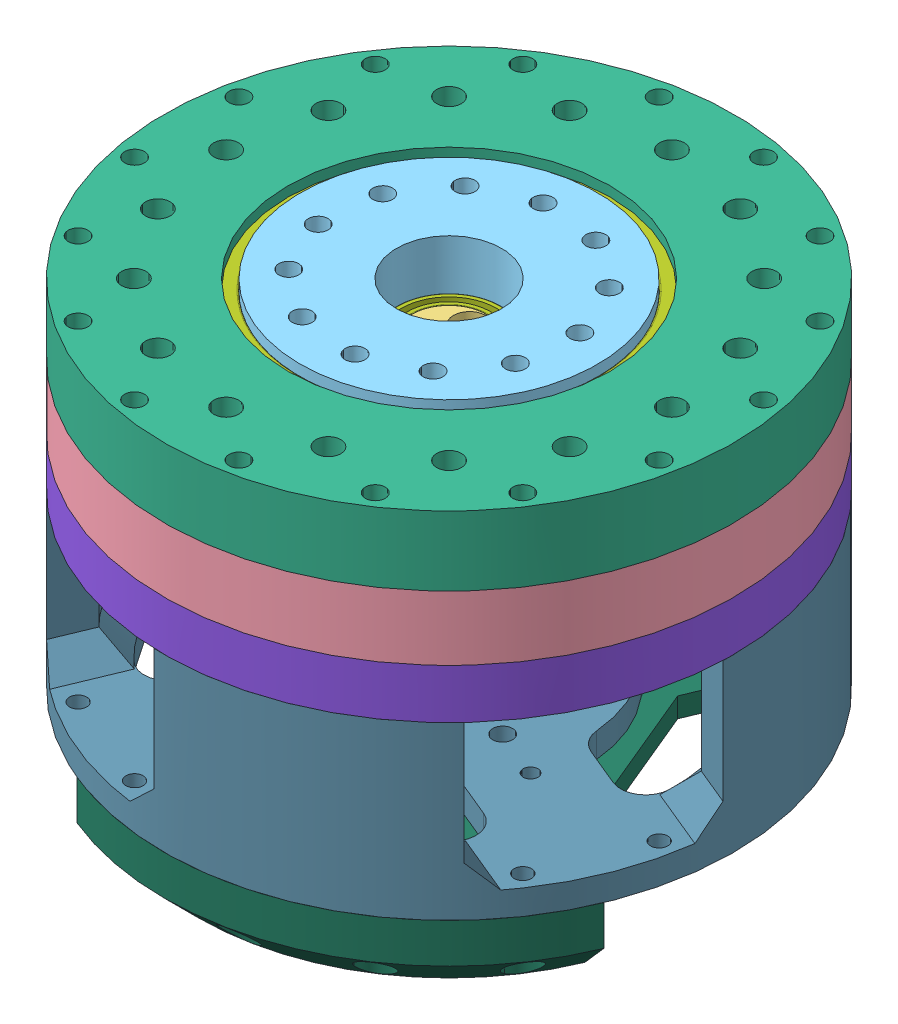
SolidWorks assembly Cycloidal, configuration Default. Lengths in mm.
Overall size (162.63 86.6 162.63).
91 component instances, 15 part files, 83 mates.
Components (placement in the parent):
- motor-X83008S.stp-1: motor-X83008S.stp [Default] at (44.8559 83.3915 132.8566) x (-0.221421 0 -0.975178) z (0 -1 0) (suppressed, hidden)
- Base_Plate-1: Base_Plate [Default] at (47.267 63.2573 89.1587) x (-0.03427 0 0.999413) z (-0.999413 0 -0.03427) size (39.8 11 39.8)
- Eccentric_Shaft-1: Eccentric_Shaft [Default] at (54.4098 67.9165 103.5023) x (-0.999413 0 -0.03427) z (0.03427 0 -0.999413) size (20 17 17)
  - Eccentric_Shaft_bot-1: Eccentric_Shaft_bot [Default] at (7.6302 12.3409 14.0904) x (1 0 0) z (0 0 -1) size (17 6 17)
  - Eccentric_Shaft_bot-2: Eccentric_Shaft_bot [Default] at (7.6302 12.3409 14.0904) x (-1 0 0) z (0 0 -1) size (17 6 17)
  - Eccentric_Shaft_top-1: Eccentric_Shaft_top [Default] at (7.6302 18.3409 14.0904) x (-1 0 0) z (0 0 -1) size (17 5 17)
- Ring_Pin_Housing-1: Ring_Pin_Housing [Default] at (47.267 74.2573 89.1587) x (0.707107 0 -0.707107) z (0.707107 0 0.707107) size (115 13 115)
- Output_Shaft-1: Output_Shaft [Default] at (47.267 87.2573 89.1587) x (0.353379 0 -0.93548) z (0.93548 0 0.353379) size (70 14 70)
- Cover-1: Cover [Default] at (47.267 87.2573 89.1587) x (0.707107 0 -0.707107) z (0.707107 0 0.707107) size (115 14.4 115)
- radial ball bearing_68_iso-39: radial ball bearing_68_iso [ISO 15 RBB - 1860 - 32,SI,NC,32_68] at (47.267 94.2573 89.1587) x (0 1 0) z (-0.131235 0 0.991351) size (10 78 78)
- radial ball bearing_68_iso-40: radial ball bearing_68_iso [ISO 15 RBB - 1840 - 32,SI,NC,32_68] at (47.267 70.7573 89.1587) x (0 1 0) z (0.001003 0 0.999999) size (7 52 52)
- Base_plate_2-1: Base_plate_2 [Default] at (47.267 64.2573 89.1587) x (0.707107 0 -0.707107) z (0.707107 0 0.707107) size (115 10 115)
- m13_bearing-31: m13_bearing [Default] at (-10.7414 95.4081 67.0593) x (0.227678 0 0.973736) z (0.973736 0 -0.227678) size (13 16 13)
  - m6-1: m6 [Default] at (8.4921 2.5508 14.8914) size (6 16 6)
  - radial ball bearing_68_iso-1: radial ball bearing_68_iso [ISO 15 RBB - 286 - 10,SI,NC,10_68] at (8.4921 16.0508 14.8914) x (0 1 0) z (0 0 1) size (5 13 13)
  - radial ball bearing_68_iso-2: radial ball bearing_68_iso [ISO 15 RBB - 286 - 10,SI,NC,10_68] at (8.4921 11.0508 14.8914) x (0 1 0) z (0 0 1) size (5 13 13)
- m13_bearing-32: m13_bearing [Default] at (-14.1668 95.4081 84.2801) x (0.227678 0 0.973736) z (0.973736 0 -0.227678) size (13 16 13)
  - m6-1: m6 [Default] at (8.4921 2.5508 14.8914) size (6 16 6)
  - radial ball bearing_68_iso-1: radial ball bearing_68_iso [ISO 15 RBB - 286 - 10,SI,NC,10_68] at (8.4921 16.0508 14.8914) x (0 1 0) z (0 0 1) size (5 13 13)
  - radial ball bearing_68_iso-2: radial ball bearing_68_iso [ISO 15 RBB - 286 - 10,SI,NC,10_68] at (8.4921 11.0508 14.8914) x (0 1 0) z (0 0 1) size (5 13 13)
- m13_bearing-34: m13_bearing [Default] at (13.6125 95.5581 125.8547) x (0.227678 0 0.973736) z (0.973736 0 -0.227678) size (13 16 13)
  - m6-1: m6 [Default] at (8.4921 2.5508 14.8914) size (6 16 6)
  - radial ball bearing_68_iso-1: radial ball bearing_68_iso [ISO 15 RBB - 286 - 10,SI,NC,10_68] at (8.4921 16.0508 14.8914) x (0 1 0) z (0 0 1) size (5 13 13)
  - radial ball bearing_68_iso-2: radial ball bearing_68_iso [ISO 15 RBB - 286 - 10,SI,NC,10_68] at (8.4921 11.0508 14.8914) x (0 1 0) z (0 0 1) size (5 13 13)
- m13_bearing-35: m13_bearing [Default] at (-0.9866 95.4081 116.0999) x (0.227678 0 0.973736) z (0.973736 0 -0.227678) size (13 16 13)
  - m6-1: m6 [Default] at (8.4921 2.5508 14.8914) size (6 16 6)
  - radial ball bearing_68_iso-1: radial ball bearing_68_iso [ISO 15 RBB - 286 - 10,SI,NC,10_68] at (8.4921 16.0508 14.8914) x (0 1 0) z (0 0 1) size (5 13 13)
  - radial ball bearing_68_iso-2: radial ball bearing_68_iso [ISO 15 RBB - 286 - 10,SI,NC,10_68] at (8.4921 11.0508 14.8914) x (0 1 0) z (0 0 1) size (5 13 13)
- m13_bearing-36: m13_bearing [Default] at (-10.7414 95.5581 101.5009) x (0.227678 0 0.973736) z (0.973736 0 -0.227678) size (13 16 13)
  - m6-1: m6 [Default] at (8.4921 2.5508 14.8914) size (6 16 6)
  - radial ball bearing_68_iso-1: radial ball bearing_68_iso [ISO 15 RBB - 286 - 10,SI,NC,10_68] at (8.4921 16.0508 14.8914) x (0 1 0) z (0 0 1) size (5 13 13)
  - radial ball bearing_68_iso-2: radial ball bearing_68_iso [ISO 15 RBB - 286 - 10,SI,NC,10_68] at (8.4921 11.0508 14.8914) x (0 1 0) z (0 0 1) size (5 13 13)
- m13_bearing-1: m13_bearing [Default] at (-0.8801 95.4081 62.5627) x (0.736525 0 0.676411) z (0.676411 0 -0.736525) size (13 16 13)
  - m6-1: m6 [Default] at (8.4921 2.5508 14.8914) size (6 16 6)
  - radial ball bearing_68_iso-1: radial ball bearing_68_iso [ISO 15 RBB - 286 - 10,SI,NC,10_68] at (8.4921 16.0508 14.8914) x (0 1 0) z (0 0 1) size (5 13 13)
  - radial ball bearing_68_iso-2: radial ball bearing_68_iso [ISO 15 RBB - 286 - 10,SI,NC,10_68] at (8.4921 11.0508 14.8914) x (0 1 0) z (0 0 1) size (5 13 13)
- m13_bearing-2: m13_bearing [Default] at (48.6831 95.4081 124.0939) x (0.120271 0 0.992741) z (0.992741 0 -0.120271) size (13 16 13)
  - m6-1: m6 [Default] at (8.4921 2.5508 14.8914) size (6 16 6)
  - radial ball bearing_68_iso-1: radial ball bearing_68_iso [ISO 15 RBB - 286 - 10,SI,NC,10_68] at (8.4921 16.0508 14.8914) x (0 1 0) z (0 0 1) size (5 13 13)
  - radial ball bearing_68_iso-2: radial ball bearing_68_iso [ISO 15 RBB - 286 - 10,SI,NC,10_68] at (8.4921 11.0508 14.8914) x (0 1 0) z (0 0 1) size (5 13 13)
- m13_bearing-3: m13_bearing [Default] at (32.7832 95.4081 34.9886) x (-0.046141 0 0.998935) z (0.998935 0 0.046141) size (13 16 13)
  - m6-1: m6 [Default] at (8.4921 2.5508 14.8914) size (6 16 6)
  - radial ball bearing_68_iso-1: radial ball bearing_68_iso [ISO 15 RBB - 286 - 10,SI,NC,10_68] at (8.4921 16.0508 14.8914) x (0 1 0) z (0 0 1) size (5 13 13)
  - radial ball bearing_68_iso-2: radial ball bearing_68_iso [ISO 15 RBB - 286 - 10,SI,NC,10_68] at (8.4921 11.0508 14.8914) x (0 1 0) z (0 0 1) size (5 13 13)
- m13_bearing-4: m13_bearing [Default] at (77.1902 95.4081 81.0003) x (0.022268 0 0.999752) z (0.999752 0 -0.022268) size (13 16 13)
  - m6-1: m6 [Default] at (8.4921 2.5508 14.8914) size (6 16 6)
  - radial ball bearing_68_iso-1: radial ball bearing_68_iso [ISO 15 RBB - 286 - 10,SI,NC,10_68] at (8.4921 16.0508 14.8914) x (0 1 0) z (0 0 1) size (5 13 13)
  - radial ball bearing_68_iso-2: radial ball bearing_68_iso [ISO 15 RBB - 286 - 10,SI,NC,10_68] at (8.4921 11.0508 14.8914) x (0 1 0) z (0 0 1) size (5 13 13)
- m13_bearing-5: m13_bearing [Default] at (73.474 95.4081 98.7828) x (0.059133 0 0.99825) z (0.99825 0 -0.059133) size (13 16 13)
  - m6-1: m6 [Default] at (8.4921 2.5508 14.8914) size (6 16 6)
  - radial ball bearing_68_iso-1: radial ball bearing_68_iso [ISO 15 RBB - 286 - 10,SI,NC,10_68] at (8.4921 16.0508 14.8914) x (0 1 0) z (0 0 1) size (5 13 13)
  - radial ball bearing_68_iso-2: radial ball bearing_68_iso [ISO 15 RBB - 286 - 10,SI,NC,10_68] at (8.4921 11.0508 14.8914) x (0 1 0) z (0 0 1) size (5 13 13)
- m13_bearing-6: m13_bearing [Default] at (12.9248 95.4081 46.7315) x (0.451561 0 0.89224) z (0.89224 0 -0.451561) size (13 16 13)
  - m6-1: m6 [Default] at (8.4921 2.5508 14.8914) size (6 16 6)
  - radial ball bearing_68_iso-1: radial ball bearing_68_iso [ISO 15 RBB - 286 - 10,SI,NC,10_68] at (8.4921 16.0508 14.8914) x (0 1 0) z (0 0 1) size (5 13 13)
  - radial ball bearing_68_iso-2: radial ball bearing_68_iso [ISO 15 RBB - 286 - 10,SI,NC,10_68] at (8.4921 11.0508 14.8914) x (0 1 0) z (0 0 1) size (5 13 13)
- m13_bearing-7: m13_bearing [Default] at (56.6452 95.4081 32.3406) x (-0.545813 0 0.837907) z (0.837907 0 0.545813) size (13 16 13)
  - m6-1: m6 [Default] at (8.4921 2.5508 14.8914) size (6 16 6)
  - radial ball bearing_68_iso-1: radial ball bearing_68_iso [ISO 15 RBB - 286 - 10,SI,NC,10_68] at (8.4921 16.0508 14.8914) x (0 1 0) z (0 0 1) size (5 13 13)
  - radial ball bearing_68_iso-2: radial ball bearing_68_iso [ISO 15 RBB - 286 - 10,SI,NC,10_68] at (8.4921 11.0508 14.8914) x (0 1 0) z (0 0 1) size (5 13 13)
- m13_bearing-8: m13_bearing [Default] at (63.0373 95.4081 51.3153) x (0.158553 0 0.98735) z (0.98735 0 -0.158553) size (13 16 13)
  - m6-1: m6 [Default] at (8.4921 2.5508 14.8914) size (6 16 6)
  - radial ball bearing_68_iso-1: radial ball bearing_68_iso [ISO 15 RBB - 286 - 10,SI,NC,10_68] at (8.4921 16.0508 14.8914) x (0 1 0) z (0 0 1) size (5 13 13)
  - radial ball bearing_68_iso-2: radial ball bearing_68_iso [ISO 15 RBB - 286 - 10,SI,NC,10_68] at (8.4921 11.0508 14.8914) x (0 1 0) z (0 0 1) size (5 13 13)
- m13_bearing-9: m13_bearing [Default] at (83.8577 95.4081 55.5358) x (-0.687134 0 0.72653) z (0.72653 0 0.687134) size (13 16 13)
  - m6-1: m6 [Default] at (8.4921 2.5508 14.8914) size (6 16 6)
  - radial ball bearing_68_iso-1: radial ball bearing_68_iso [ISO 15 RBB - 286 - 10,SI,NC,10_68] at (8.4921 16.0508 14.8914) x (0 1 0) z (0 0 1) size (5 13 13)
  - radial ball bearing_68_iso-2: radial ball bearing_68_iso [ISO 15 RBB - 286 - 10,SI,NC,10_68] at (8.4921 11.0508 14.8914) x (0 1 0) z (0 0 1) size (5 13 13)
- m13_bearing-11: m13_bearing [Default] at (30.1977 95.4081 135.7424) x (0.57351 0 0.819198) z (0.819198 0 -0.57351) size (13 16 13)
  - m6-1: m6 [Default] at (8.4921 2.5508 14.8914) size (6 16 6)
  - radial ball bearing_68_iso-1: radial ball bearing_68_iso [ISO 15 RBB - 286 - 10,SI,NC,10_68] at (8.4921 16.0508 14.8914) x (0 1 0) z (0 0 1) size (5 13 13)
  - radial ball bearing_68_iso-2: radial ball bearing_68_iso [ISO 15 RBB - 286 - 10,SI,NC,10_68] at (8.4921 11.0508 14.8914) x (0 1 0) z (0 0 1) size (5 13 13)
- m13_bearing-12: m13_bearing [Default] at (62.8861 95.4081 115.3744) x (0.184178 0 0.982893) z (0.982893 0 -0.184178) size (13 16 13)
  - m6-1: m6 [Default] at (8.4921 2.5508 14.8914) size (6 16 6)
  - radial ball bearing_68_iso-1: radial ball bearing_68_iso [ISO 15 RBB - 286 - 10,SI,NC,10_68] at (8.4921 16.0508 14.8914) x (0 1 0) z (0 0 1) size (5 13 13)
  - radial ball bearing_68_iso-2: radial ball bearing_68_iso [ISO 15 RBB - 286 - 10,SI,NC,10_68] at (8.4921 11.0508 14.8914) x (0 1 0) z (0 0 1) size (5 13 13)
- M3x4x4.2_brass_insert-22: M3x4x4.2_brass_insert [Default] at (47.1299 63.2573 93.1563) x (0.984609 0 -0.174769) z (0.174769 0 0.984609) size (4 4 4)
- M3x4x4.2_brass_insert-23: M3x4x4.2_brass_insert [Default] at (47.4041 63.2573 85.161) x (0.984609 0 -0.174769) z (0.174769 0 0.984609) size (4 4 4)
- radial ball bearing_68_iso-44: radial ball bearing_68_iso [ISO 15 RBB - 1715 - 26,SI,NC,26_68] at (45.7679 83.7573 89.1073) x (0 1 0) z (-0.714953 0 -0.699173) size (4 21 21)
- radial ball bearing_68_iso-45: radial ball bearing_68_iso [ISO 15 RBB - 1715 - 26,SI,NC,26_68] at (47.267 89.2573 89.1587) x (0 1 0) z (0.999483 0 -0.032163) size (4 21 21)
- radial ball bearing_68_iso-46: radial ball bearing_68_iso [ISO 15 RBB - 1715 - 26,SI,NC,26_68] at (48.7661 76.2573 89.2101) x (0 -1 0) z (0.546944 0 -0.837169) size (4 21 21)
- socket button head screw_iso-37: socket button head screw_iso [ISO 7380 - M4 x 12 - 12N] at (79.0868 62.0573 57.3389) x (0 1 0) z (-0.709975 0 0.704227) size (14.2 7.6 7.6)
- socket button head screw_iso-38: socket button head screw_iso [ISO 7380 - M4 x 12 - 12N] at (64.4877 62.0573 130.7332) x (0 1 0) z (-0.724148 0 0.689645) size (14.2 7.6 7.6)
- foc-motor-controller.step-1: foc-motor-controller.step [Default] at (47.267 27.2573 89.1587) x (0.382683 0 0.92388) z (0 -1 0) (suppressed, hidden)
- hex nut style 1 gradeab_iso-1: hex nut style 1 gradeab_iso [ISO - 4032 - M3 - W - N] at (58.9027 27.2573 61.0676) x (1 0 0) z (0 -1 0) size (5.5 6.35 2.4)
- Cycloidal_Discs_8308-1: Cycloidal_Discs_8308 [Default] at (-23.7878 41.227 91.2662) x (0.524326 0 -0.851518) z (0.851518 0 0.524326) size (79.25 5 79.73)
  - Cycloidal_Discs-1: Cycloidal_Discs [Default] at (38.3081 39.5303 58.0959) size (79.25 5 79.73)
- Cycloidal_Discs_8308-2: Cycloidal_Discs_8308 [Default] at (10.472 118.7876 147.3152) x (1 0 -0.000242) z (-0.000242 0 -1) size (79.25 5 79.73)
  - Cycloidal_Discs-1: Cycloidal_Discs [Default] at (38.3081 39.5303 58.0959) size (79.25 5 79.73)
- Motor_Cover_v2-2: Motor_Cover_v2 [Default] at (47.267 29.6573 89.1587) x (0.92388 0 0.382683) z (-0.382683 0 0.92388) size (115 34.6 115)
- driver_cover-1: driver_cover [Default] at (47.267 29.6573 89.1587) x (0.92321 0 -0.384295) z (-0.384295 0 -0.92321) size (81.32 15 115)
Mates (geometry in assembly coordinates):
- Coincident1: coincident anti-aligned: plane of motor-X83008S.stp-1/outrunner.stp-1 through (81.7467 63.2573 90.341) normal (0 1 0); plane of Base_Plate-1 through (47.267 63.2573 89.1587) normal (0 -1 0)
- Concentric1: concentric anti-aligned: line of motor-X83008S.stp-1/outrunner.stp-1 through (62.7579 57.7573 89.6899) axis (0 1 0); cylinder of Base_Plate-1 through (62.7579 74.2573 89.6899) axis (0 -1 0) radius 2
- Concentric2: concentric anti-aligned: cylinder of motor-X83008S.stp-1/shaft.stp-1 through (47.267 63.2573 89.1587) axis (0 1 0) radius 1.5; line of Base_Plate-1 through (47.267 74.2573 89.1587) axis (0 -1 0)
- Concentric75: concentric anti-aligned: cylinder of Output_Shaft-1 through (47.267 101.2573 89.1587) axis (0 -1 0) radius 30; cylinder of radial ball bearing_68_iso-39 through (47.267 73.6198 89.1587) axis (0 1 0) radius 30
- Concentric76: concentric anti-aligned: cylinder of Cover-1 through (47.267 99.2573 89.1587) axis (0 -1 0) radius 39; cylinder of radial ball bearing_68_iso-39 through (47.267 73.6198 89.1587) axis (0 1 0) radius 39
- Concentric78: concentric anti-aligned: cylinder of Base_Plate-1 through (47.267 74.2573 89.1587) axis (0 -1 0) radius 19.9; cylinder of radial ball bearing_68_iso-40 through (47.267 50.1198 89.1587) axis (0 1 0) radius 20
- Concentric79: concentric aligned: cylinder of Ring_Pin_Housing-1 through (2.3676 87.2573 59.1579) axis (0 -1 0) radius 1.6; cylinder of Base_plate_2-1 through (2.3676 74.2573 59.1579) axis (0 -1 0) radius 1.75
- Concentric80: concentric aligned: cylinder of Ring_Pin_Housing-1 through (47.267 87.2573 89.1587) axis (0 -1 0) radius 57.5; cylinder of Base_plate_2-1 through (47.267 74.2573 89.1587) axis (0 -1 0) radius 57.5
- Coincident107: coincident anti-aligned: plane of Ring_Pin_Housing-1 through (47.267 74.2573 89.1587) normal (0 -1 0); plane of Base_plate_2-1 through (47.267 74.2573 89.1587) normal (0 1 0)
- Concentric83: concentric aligned: cylinder of Ring_Pin_Housing-1 through (2.3676 87.2573 59.1579) axis (0 -1 0) radius 1.6; cylinder of Cover-1 through (2.3676 99.2573 59.1579) axis (0 -1 0) radius 2
- Concentric84: concentric aligned: cylinder of Cover-1 through (15.4472 89.2573 57.3389) axis (0 1 0) radius 2.5; cylinder of m13_bearing-1/m6-1 through (15.4472 86.8573 57.3389) axis (0 1 0) radius 2
- Concentric85: concentric aligned: cylinder of Cover-1 through (47.267 89.2573 134.1587) axis (0 1 0) radius 2.5; cylinder of m13_bearing-11/m6-1 through (47.267 86.8573 134.1587) axis (0 1 0) radius 2
- Concentric86: concentric aligned: cylinder of Cover-1 through (64.4877 89.2573 130.7332) axis (0 1 0) radius 2.5; cylinder of m13_bearing-2/m6-1 through (64.4877 86.8573 130.7332) axis (0 1 0) radius 2
- Concentric87: concentric aligned: cylinder of Cover-1 through (79.0868 89.2573 120.9785) axis (0 1 0) radius 2.5; cylinder of m13_bearing-12/m6-1 through (79.0868 86.8573 120.9785) axis (0 1 0) radius 2
- Concentric88: concentric aligned: cylinder of Cover-1 through (88.8416 89.2573 106.3794) axis (0 1 0) radius 2.5; cylinder of m13_bearing-5/m6-1 through (88.8416 86.8573 106.3794) axis (0 1 0) radius 2
- Concentric89: concentric aligned: cylinder of Cover-1 through (92.267 89.2573 89.1587) axis (0 1 0) radius 2.5; cylinder of m13_bearing-4/m6-1 through (92.267 86.8573 89.1587) axis (0 1 0) radius 2
- Concentric90: concentric aligned: cylinder of Cover-1 through (30.0462 89.2573 47.5841) axis (0 1 0) radius 2.5; cylinder of m13_bearing-6/m6-1 through (30.0462 86.8573 47.5841) axis (0 1 0) radius 2
- Concentric91: concentric aligned: cylinder of Cover-1 through (47.267 89.2573 44.1587) axis (0 1 0) radius 2.5; cylinder of m13_bearing-3/m6-1 through (47.267 86.8573 44.1587) axis (0 1 0) radius 2
- Concentric92: concentric aligned: cylinder of Cover-1 through (64.4877 89.2573 47.5841) axis (0 1 0) radius 2.5; cylinder of m13_bearing-7/m6-1 through (64.4877 86.8573 47.5841) axis (0 1 0) radius 2
- Concentric93: concentric aligned: cylinder of Cover-1 through (79.0868 89.2573 57.3389) axis (0 1 0) radius 2.5; cylinder of m13_bearing-8/m6-1 through (79.0868 86.8573 57.3389) axis (0 1 0) radius 2
- Concentric94: concentric aligned: cylinder of Cover-1 through (88.8416 89.2573 71.9379) axis (0 1 0) radius 2.5; cylinder of m13_bearing-9/m6-1 through (88.8416 86.8573 71.9379) axis (0 1 0) radius 2
- Coincident132: coincident anti-aligned: plane of Ring_Pin_Housing-1 through (47.267 87.2573 89.1587) normal (0 1 0); plane of Cover-1 through (47.267 87.2573 89.1587) normal (0 -1 0)
- Concentric1437: concentric anti-aligned: cylinder of Base_Plate-1 through (47.1299 74.2573 93.1563) axis (0 -1 0) radius 2; cylinder of M3x4x4.2_brass_insert-22 through (47.1299 68.1594 93.1563) axis (0 1 0) radius 1.5
- Coincident1479: coincident aligned: plane of Base_Plate-1 through (47.267 63.2573 89.1587) normal (0 -1 0); plane of M3x4x4.2_brass_insert-22 through (48.6068 63.2573 92.8942) normal (0 -1 0)
- Concentric1438: concentric anti-aligned: cylinder of Base_Plate-1 through (47.4041 74.2573 85.161) axis (0 -1 0) radius 2; cylinder of M3x4x4.2_brass_insert-23 through (47.4041 68.1594 85.161) axis (0 1 0) radius 1.5
- Coincident1480: coincident aligned: plane of Base_Plate-1 through (47.267 63.2573 89.1587) normal (0 -1 0); plane of M3x4x4.2_brass_insert-23 through (48.881 63.2573 84.8989) normal (0 -1 0)
- Coincident1486632: coincident anti-aligned: plane of Cover-1 through (88.8416 86.8573 71.9379) normal (0 -1 0); plane of m13_bearing-9/radial ball bearing_68_iso-2 through (91.6245 86.8573 68.9955) normal (0 1 0)
- Coincident1486633: coincident anti-aligned: plane of Cover-1 through (88.8416 86.8573 71.9379) normal (0 -1 0); plane of m13_bearing-8/radial ball bearing_68_iso-2 through (78.4447 86.8573 53.3401) normal (0 1 0)
- Coincident1486634: coincident anti-aligned: plane of Cover-1 through (88.8416 86.8573 71.9379) normal (0 -1 0); plane of m13_bearing-7/radial ball bearing_68_iso-2 through (66.6983 86.8573 44.1906) normal (0 1 0)
- Coincident1486635: coincident anti-aligned: plane of Cover-1 through (88.8416 86.8573 71.9379) normal (0 -1 0); plane of m13_bearing-3/radial ball bearing_68_iso-2 through (47.4539 86.8573 40.113) normal (0 1 0)
- Coincident1486636: coincident anti-aligned: plane of Cover-1 through (88.8416 86.8573 71.9379) normal (0 -1 0); plane of m13_bearing-4/radial ball bearing_68_iso-2 through (92.1768 86.8573 85.1097) normal (0 1 0)
- Coincident1486637: coincident anti-aligned: plane of Cover-1 through (88.8416 86.8573 71.9379) normal (0 -1 0); plane of m13_bearing-5/radial ball bearing_68_iso-2 through (88.6021 86.8573 102.3365) normal (0 1 0)
- Coincident1486638: coincident anti-aligned: plane of Cover-1 through (88.8416 86.8573 71.9379) normal (0 -1 0); plane of m13_bearing-12/radial ball bearing_68_iso-2 through (78.3409 86.8573 116.9978) normal (0 1 0)
- Coincident1486639: coincident anti-aligned: plane of Cover-1 through (88.8416 86.8573 71.9379) normal (0 -1 0); plane of m13_bearing-11/radial ball bearing_68_iso-2 through (44.9443 86.8573 130.8409) normal (0 1 0)
- Coincident1486640: coincident anti-aligned: plane of Cover-1 through (88.8416 86.8573 71.9379) normal (0 -1 0); plane of m13_bearing-2/radial ball bearing_68_iso-2 through (64.0006 86.8573 126.7126) normal (0 1 0)
- Coincident1486643: coincident anti-aligned: plane of Cover-1 through (30.0462 86.8573 47.5841) normal (0 -1 0); plane of m13_bearing-6/radial ball bearing_68_iso-2 through (28.2174 86.8573 43.9705) normal (0 1 0)
- Coincident1486644: coincident anti-aligned: plane of Cover-1 through (15.4472 86.8573 57.3389) normal (0 -1 0); plane of m13_bearing-1/radial ball bearing_68_iso-2 through (12.4643 86.8573 54.5994) normal (0 1 0)
- Concentric1445035: concentric anti-aligned: cylinder of Eccentric_Shaft-1/Eccentric_Shaft_bot-1 through (48.7661 74.2573 89.2101) axis (0 1 0) radius 7.5; cylinder of radial ball bearing_68_iso-46 through (48.7661 96.8948 89.2101) axis (0 -1 0) radius 7.5
- Coincident1486648: coincident aligned: plane of Eccentric_Shaft-1/Eccentric_Shaft_bot-1 through (48.7661 74.2573 89.2101) normal (0 -1 0); plane of radial ball bearing_68_iso-46 through (42.3199 74.2573 84.9986) normal (0 -1 0)
- Concentric1445036: concentric anti-aligned: cylinder of Eccentric_Shaft-1/Eccentric_Shaft_bot-2 through (45.7679 86.2573 89.1073) axis (0 -1 0) radius 7.5; cylinder of radial ball bearing_68_iso-44 through (45.7679 63.1198 89.1073) axis (0 1 0) radius 7.5
- Coincident1486649: coincident aligned: plane of Eccentric_Shaft-1/Eccentric_Shaft_bot-2 through (45.7679 81.7573 89.1073) normal (0 1 0); circle of radial ball bearing_68_iso-44
- Concentric1445037: concentric anti-aligned: cylinder of Eccentric_Shaft-1/Eccentric_Shaft_top-1 through (47.267 91.2573 89.1587) axis (0 -1 0) radius 7.5; cylinder of radial ball bearing_68_iso-45 through (47.267 68.6198 89.1587) axis (0 1 0) radius 7.5
- Concentric1445038: concentric anti-aligned: cylinder of Base_Plate-1 through (47.267 74.2573 89.1587) axis (0 -1 0) radius 19.9; cylinder of radial ball bearing_68_iso-40 through (47.267 50.1198 89.1587) axis (0 1 0) radius 20
- Coincident1486651: coincident aligned: plane of Base_Plate-1 through (47.267 74.2573 89.1587) normal (0 1 0); plane of Base_plate_2-1 through (47.267 74.2573 89.1587) normal (0 1 0)
- Concentric1445041: concentric anti-aligned: cylinder of radial ball bearing_68_iso-40 through (47.267 50.1198 89.1587) axis (0 1 0) radius 26; cylinder of Base_plate_2-1 through (47.267 74.2573 89.1587) axis (0 -1 0) radius 26.1
- Coincident1486655: coincident anti-aligned: plane of Eccentric_Shaft-1/Eccentric_Shaft_top-1 through (47.267 87.2573 89.1587) normal (0 1 0); plane of radial ball bearing_68_iso-45 through (47.5372 87.2573 97.5543) normal (0 -1 0)
- Concentric1445042: concentric aligned: cylinder of Base_Plate-1 through (47.4041 74.2573 85.161) axis (0 -1 0) radius 2; cylinder of Eccentric_Shaft-1/Eccentric_Shaft_bot-1 through (47.4041 80.2573 85.161) axis (0 -1 0) radius 1.6
- Concentric1445043: concentric anti-aligned: cylinder of Eccentric_Shaft-1/Eccentric_Shaft_bot-1 through (47.1299 80.2573 93.1563) axis (0 -1 0) radius 1.6; cylinder of M3x4x4.2_brass_insert-22 through (47.1299 68.1594 93.1563) axis (0 1 0) radius 1.5
- Concentric1445044: concentric aligned: cylinder of Base_plate_2-1 through (79.0868 74.2573 57.3389) axis (0 -1 0) radius 2.1; cylinder of socket button head screw_iso-37 through (79.0868 62.0573 57.3389) axis (0 -1 0) radius 2
- Coincident1486656: coincident anti-aligned: plane of Base_plate_2-1 through (47.267 64.2573 89.1587) normal (0 -1 0); plane of socket button head screw_iso-37 through (77.6783 64.2573 55.9189) normal (0 1 0)
- Concentric1445045: concentric aligned: cylinder of Base_plate_2-1 through (64.4877 74.2573 130.7332) axis (0 -1 0) radius 2.1; cylinder of socket button head screw_iso-38 through (64.4877 62.0573 130.7332) axis (0 -1 0) radius 2
- Coincident1486657: coincident anti-aligned: plane of Base_plate_2-1 through (47.267 64.2573 89.1587) normal (0 -1 0); plane of socket button head screw_iso-38 through (63.1085 64.2573 129.285) normal (0 1 0)
- Coincident1486660: coincident aligned: plane of Cover-1 through (5.6924 86.8573 71.9379) normal (0 -1 0); circle of m13_bearing-31/radial ball bearing_68_iso-2
- Coincident1486661: coincident aligned: plane of Cover-1 through (5.6924 86.8573 71.9379) normal (0 -1 0); circle of m13_bearing-32/radial ball bearing_68_iso-2
- Coincident1486662: coincident aligned: plane of Cover-1 through (5.6924 86.8573 71.9379) normal (0 -1 0); circle of m13_bearing-36/radial ball bearing_68_iso-2
- Coincident1486663: coincident aligned: plane of Cover-1 through (5.6924 86.8573 71.9379) normal (0 -1 0); circle of m13_bearing-35/radial ball bearing_68_iso-2
- Coincident1486664: coincident aligned: plane of Cover-1 through (5.6924 86.8573 71.9379) normal (0 -1 0); circle of m13_bearing-34/radial ball bearing_68_iso-2
- Concentric1445057: concentric aligned: cylinder of Base_plate_2-1 through (5.6924 74.2573 71.9379) axis (0 -1 0) radius 2.1; cylinder of m13_bearing-31/radial ball bearing_68_iso-2 through (5.6924 104.9948 71.9379) axis (0 -1 0) radius 6.5
- Concentric1445058: concentric aligned: cylinder of Ring_Pin_Housing-1 through (2.267 87.2573 89.1587) axis (0 -1 0) radius 7; cylinder of m13_bearing-32/radial ball bearing_68_iso-2 through (2.267 104.9948 89.1587) axis (0 -1 0) radius 6.5
- Concentric1445059: concentric aligned: cylinder of Ring_Pin_Housing-1 through (5.6924 87.2573 106.3794) axis (0 -1 0) radius 7; cylinder of m13_bearing-36/radial ball bearing_68_iso-2 through (5.6924 105.1448 106.3794) axis (0 -1 0) radius 6.5
- Concentric1445060: concentric aligned: cylinder of Ring_Pin_Housing-1 through (15.4472 87.2573 120.9785) axis (0 -1 0) radius 7; cylinder of m13_bearing-35/radial ball bearing_68_iso-2 through (15.4472 104.9948 120.9785) axis (0 -1 0) radius 6.5
- Concentric1445061: concentric aligned: cylinder of Ring_Pin_Housing-1 through (30.0462 87.2573 130.7332) axis (0 -1 0) radius 7; cylinder of m13_bearing-34/radial ball bearing_68_iso-2 through (30.0462 105.1448 130.7332) axis (0 -1 0) radius 6.5
- Coincident1486692: coincident anti-aligned: plane of foc-motor-controller.step-1/foc-motor-controller_PCB.step-1 through (47.267 27.2573 89.1587) normal (0 1 0); plane of hex nut style 1 gradeab_iso-1 through (58.9027 27.2573 64.243) normal (0 -1 0)
- Concentric14450545: concentric anti-aligned: cylinder of radial ball bearing_68_iso-46 through (48.7661 96.8948 89.2101) axis (0 -1 0) radius 10.5; cylinder of Cycloidal_Discs_8308-2/Cycloidal_Discs-1 through (48.7661 74.2573 89.2101) axis (0 1 0) radius 10.6
- Coincident1486693: coincident aligned: plane of radial ball bearing_68_iso-46 through (40.1433 74.2573 83.5766) normal (0 -1 0); plane of Cycloidal_Discs_8308-2/Cycloidal_Discs-1 through (48.9427 74.2573 127.5714) normal (0 -1 0)
- Concentric14450546: concentric anti-aligned: cylinder of radial ball bearing_68_iso-44 through (45.7679 63.1198 89.1073) axis (0 1 0) radius 10.5; cylinder of Cycloidal_Discs_8308-1/Cycloidal_Discs-1 through (45.7679 85.7573 89.1073) axis (0 -1 0) radius 10.6
- Coincident1486694: coincident aligned: plane of radial ball bearing_68_iso-44 through (52.9693 85.7573 81.7433) normal (0 1 0); plane of Cycloidal_Discs_8308-1/Cycloidal_Discs-1 through (13.1902 85.7573 68.8509) normal (0 1 0)
- Concentric14450552: concentric aligned: cylinder of Ring_Pin_Housing-1 through (47.267 87.2573 89.1587) axis (0 -1 0) radius 57.5; cylinder of Cover-1 through (47.267 99.2573 89.1587) axis (0 -1 0) radius 57.5
- Concentric14450553: concentric aligned: cylinder of Cover-1 through (47.267 99.2573 89.1587) axis (0 -1 0) radius 57.5; cylinder of Motor_Cover_v2-2 through (47.267 64.2573 89.1587) axis (0 -1 0) radius 57.5
- Coincident1486698: coincident anti-aligned: plane of Base_plate_2-1 through (47.267 64.2573 89.1587) normal (0 -1 0); plane of Motor_Cover_v2-2 through (47.267 64.2573 89.1587) normal (0 1 0)
- Concentric14450559: concentric anti-aligned: cylinder of foc-motor-controller.step-1/foc-motor-controller_PCB.step-1 through (39.8323 27.3033 118.6413) axis (0 1 0) radius 1.6; cylinder of Motor_Cover_v2-2 through (35.6313 79.6573 117.2498) axis (0 -1 0) radius 1.5
- Concentric14450560: concentric anti-aligned: circle of foc-motor-controller.step-1/foc-motor-controller_PCB.step-1; cylinder of Motor_Cover_v2-2 through (58.9027 79.6573 61.0676) axis (0 -1 0) radius 1.5
- Coincident1486699: coincident anti-aligned: line of foc-motor-controller.step-1/foc-motor-controller_PCB.step-1 through (54.7017 25.7473 59.6761) axis (0 1 0); line of hex nut style 1 gradeab_iso-1 through (54.7017 29.4569 59.6761) axis (0 -1 0)
- Coincident1486700: coincident aligned: circle of hex nut style 1 gradeab_iso-1; plane of Motor_Cover_v2-2 through (47.267 29.6573 89.1587) normal (0 -1 0)
- Concentric14450561: concentric anti-aligned: cylinder of Motor_Cover_v2-2 through (47.267 64.2573 89.1587) axis (0 -1 0) radius 57.5; cylinder of driver_cover-1 through (47.267 14.6573 89.1587) axis (0 1 0) radius 57.5
- Coincident1486701: coincident anti-aligned: plane of Motor_Cover_v2-2 through (47.267 29.6573 89.1587) normal (0 -1 0); plane of driver_cover-1 through (47.267 29.6573 89.1587) normal (0 1 0)
- Coincident1486702: coincident aligned: plane of Base_Plate-1 through (47.267 74.2573 89.1587) normal (0 1 0); plane of Base_plate_2-1 through (47.267 74.2573 89.1587) normal (0 1 0)
- Coincident1486703: coincident aligned: plane of radial ball bearing_68_iso-40 through (21.567 74.2573 89.1845) normal (0 1 0); plane of Base_plate_2-1 through (47.267 74.2573 89.1587) normal (0 1 0)
- Coincident1486704: coincident anti-aligned: plane of Base_Plate-1 through (47.267 74.2573 89.1587) normal (0 1 0); plane of Eccentric_Shaft-1/Eccentric_Shaft_bot-1 through (48.7661 74.2573 89.2101) normal (0 -1 0)
- Coincident1486705: coincident aligned: plane of Output_Shaft-1 through (47.267 101.2573 89.1587) normal (0 1 0); plane of Cover-1 through (47.267 101.2573 89.1587) normal (0 1 0)
- Coincident1486706: coincident anti-aligned: plane of Output_Shaft-1 through (47.267 89.2573 89.1587) normal (0 1 0); plane of radial ball bearing_68_iso-39 through (11.2809 89.2573 84.3948) normal (0 -1 0)
- Concentric14450562: concentric aligned: cylinder of Motor_Cover_v2-2 through (57.8019 79.6573 142.1211) axis (0 -1 0) radius 1.75; cylinder of driver_cover-1 through (57.8019 21.6573 142.1211) axis (0 -1 0) radius 3.25
- Concentric14450563: concentric aligned: cylinder of Cover-1 through (57.8019 99.2573 142.1211) axis (0 -1 0) radius 2; cylinder of Motor_Cover_v2-2 through (57.8019 79.6573 142.1211) axis (0 -1 0) radius 1.75
